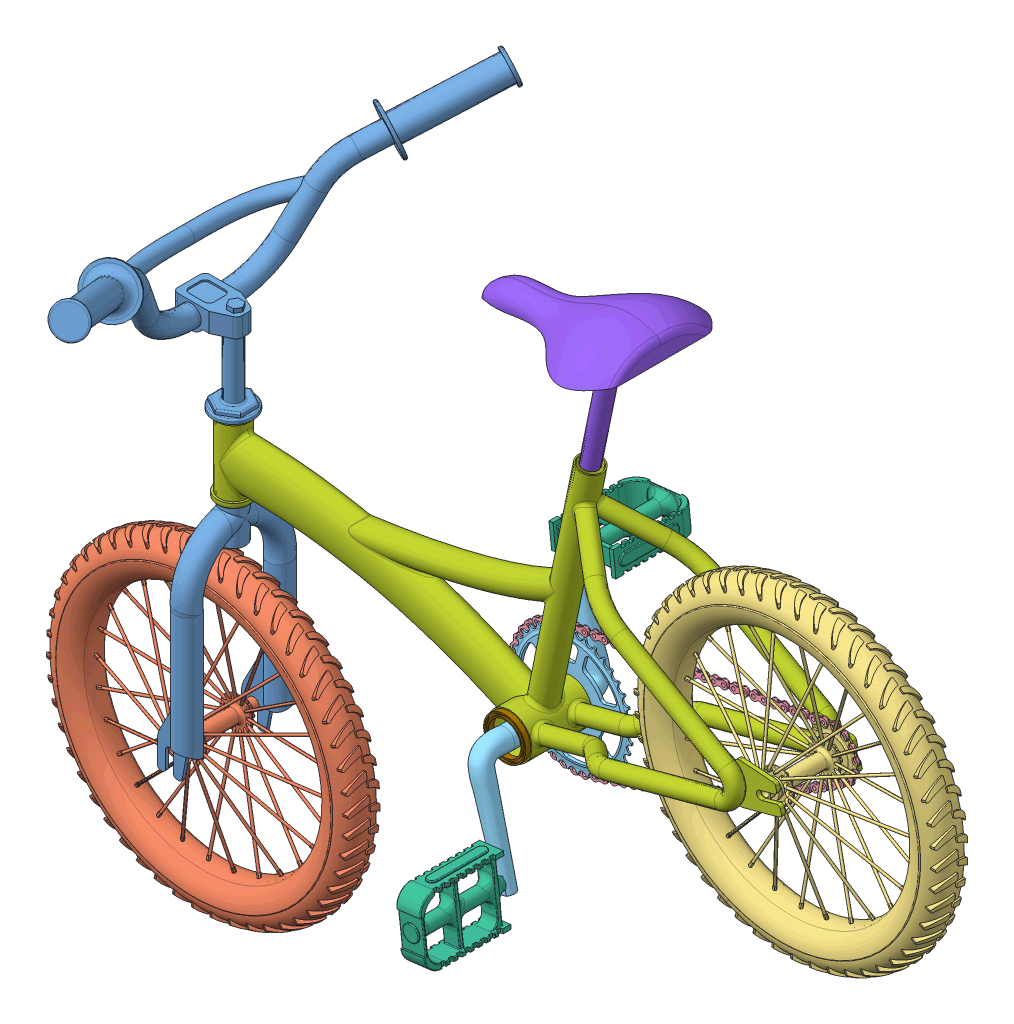
SolidWorks assembly Złożenie, configuration Domyślna. Lengths in mm.
Overall size (1253.15 963.85 568.7).
10 component instances, 9 part files, 21 mates.
Components (placement in the parent):
- Kierownica-1: Kierownica [Domyślna] at (-720.5815 -1385.0897 662.6066) size (155.77 662.61 568.7)
- Koło przód-1: Koło przód [Domyślna] at (-725.5815 -1807.8397 662.6066) x (0 0 -1) z (-0.938996 -0.343929 0) size (100 393.11 392.93)
- Koło tył-1: Koło tył [Domyślna] at (1.5514 -1492.7164 662.6066) x (0 0 -1) z (0.577742 -0.81622 0) size (89 393.11 392.93)
- Łańcuch-1: Łańcuch [Domyślna] at (-215.7289 -1502.4241 620.6066) x (-0.985639 -0.168866 0) z (0 0 -1) size (444.53 160.42 4)
- Pedał-1: Pedał [Domyślna] at (-321.3407 -1596.6109 663.6066) x (0.267848 -0.963461 0) z (0 0 1) size (270.08 150.67 176.8)
- Pedał Pedał-1: Pedał Pedał [Domyślna] at (-288.6026 -1714.6565 805.6066) x (0 0 1) z (-0.120436 0.992721 0) size (110.71 30.09 84)
- Rama-1: Rama [Domyślna] at (-226.5514 -1588.1555 662.6066) x (0.965261 0.261287 0) z (0 0 1) size (734 311.09 139.06)
- Siodełko-1: Siodełko [Domyślna] at (-272.5835 -1152.6412 662.6066) x (0.989265 0.14613 0) z (0 0 1) size (218.88 185.63 189.96)
- Pedał Pedał-2: Pedał Pedał [Domyślna] at (-354.8216 -1476.1783 521.6066) x (0 0 -1) z (-0.993951 -0.10982 0) size (110.71 30.09 84)
- instrument ball bearing_68_am-3: instrument ball bearing_68_am [AFBMA 12.1.4.1 - 0400-52 - 32,SI,NC,32_68] at (-321.3407 -1596.6109 702.9385) x (0 0 -1) z (1 0 0) size (7 52 52)
Mates (geometry in assembly coordinates):
- Wspólnie1: coincident anti-aligned: plane of Kierownica-1 through (-700.5815 -1454.0897 662.6066) normal (0 -1 0); plane of Rama-1 through (-700.5815 -1454.0897 662.6066) normal (0 1 0)
- Koncentryczne6: concentric aligned: cylinder of Kierownica-1 through (-725.5815 -1807.8397 716.6066) axis (0 0 -1) radius 5; cylinder of Koło przód-1 through (-725.5815 -1807.8397 707.1066) axis (0 0 -1) radius 7
- Szerokość1: width anti-aligned: plane of Kierownica-1 through (-708.7035 -1753.4439 608.6066) normal (0 0 -1); plane of Kierownica-1 through (-708.7035 -1753.4439 716.6066) normal (0 0 1); plane of Koło przód-1 through (-725.5815 -1807.8397 701.1066) normal (0 0 1); plane of Koło przód-1 through (-725.5815 -1807.8397 624.1066) normal (0 0 -1)
- Koncentryczne9: concentric aligned: cylinder of Koło tył-1 through (1.5514 -1492.7164 707.1066) axis (0 0 -1) radius 7; cylinder of Rama-1 through (1.5514 -1492.7164 712.6066) axis (0 0 -1) radius 5
- Szerokość2: width anti-aligned: plane of Rama-1 through (1.5514 -1492.7164 712.6066) normal (0 0 1); plane of Rama-1 through (1.5514 -1492.7164 612.6066) normal (0 0 -1); plane of Koło tył-1 through (1.5514 -1492.7164 618.1066) normal (0 0 -1); plane of Koło tył-1 through (1.5514 -1492.7164 707.1066) normal (0 0 1)
- Koncentryczne13: concentric anti-aligned: cylinder of Pedał-1 through (-321.3407 -1596.6109 706.1066) axis (0 0 -1) radius 12.5; cylinder of Rama-1 through (-321.3407 -1596.6109 593.0772) axis (0 0 1) radius 26
- Wspólnie4: coincident anti-aligned: plane of Pedał-1 through (-284.97 -1586.4997 625.1066) normal (0 0 1); plane of Rama-1 through (-321.3407 -1596.6109 625.1066) normal (0 0 -1)
- Wspólnie7: coincident anti-aligned: plane of Pedał-1 through (-429.7005 -1766.8553 745.6066) normal (0 0 1); plane of Pedał Pedał-1 through (-288.6026 -1714.6565 745.6066) normal (0 0 -1)
- Wspólnie8: coincident anti-aligned: plane of Pedał-1 through (-502.0193 -1506.7208 581.6066) normal (0 0 -1); plane of Pedał Pedał-2 through (-354.8216 -1476.1783 581.6066) normal (0 0 1)
- Stycznie4: tangent aligned: cylinder of Pedał Pedał-1 through (-288.6026 -1714.6565 755.6066) axis (0 0 1) radius 7.5; cylinder of Pedał-1 through (-287.8597 -1717.0436 513.6066) axis (0 0 1) radius 5
- Koncentryczne14: concentric anti-aligned: cylinder of Pedał-1 through (-354.8216 -1476.1783 513.6066) axis (0 0 1) radius 5; cylinder of Pedał Pedał-2 through (-354.8216 -1476.1783 571.6066) axis (0 0 -1) radius 7.5
- Koncentryczne16: concentric anti-aligned: cylinder of Kierownica-1 through (-700.5815 -1444.0897 662.6066) axis (0 -1 0) radius 15; cylinder of Rama-1 through (-700.5815 -1719.9733 662.6066) axis (0 1 0) radius 16
- Koncentryczne17: concentric aligned: cylinder of Rama-1 through (-359.7986 -1784.0089 662.6066) axis (0.201031 0.979585 0) radius 13.5; cylinder of Siodełko-1 through (-259.0211 -1292.9396 662.6066) axis (0.201031 0.979585 0) radius 10
- Równolegle5: parallel aligned: plane of Siodełko-1 through (-272.5835 -1152.6412 662.6066) normal (0 0 1)
- Wspólnie15: coincident anti-aligned: plane of Rama-1 through (-259.0211 -1292.9396 662.6066) normal (0.201031 0.979585 0); circle of Siodełko-1
- Koncentryczne18: concentric anti-aligned: circle of Łańcuch-1; circle of Pedał-1
- Wspólnie16: coincident anti-aligned: plane of Łańcuch-1 through (26.9473 -1480.8729 617.6066) normal (0 0 -1); plane of Rama-1 through (1.5514 -1492.7164 617.6066) normal (0 0 1)
- Koncentryczne23: concentric aligned: cylinder of Pedał-1 through (-321.3407 -1596.6109 706.1066) axis (0 0 -1) radius 12.5; cylinder of instrument ball bearing_68_am-3 through (-321.3407 -1596.6109 723.576) axis (0 0 -1) radius 20
- Koncentryczne24: concentric anti-aligned: cylinder of Rama-1 through (-321.3407 -1596.6109 593.0772) axis (0 0 1) radius 26; cylinder of instrument ball bearing_68_am-3 through (-321.3407 -1596.6109 723.576) axis (0 0 -1) radius 26
- Wiązanie kół zębatych1: gear = 361.1908 : 130 mm: circle of Pedał-1; circle of Koło tył-1
- Wiązanie kół zębatych2: gear = 339.8032 : 294.5498 mm: circle of Koło przód-1; circle of Koło tył-1
